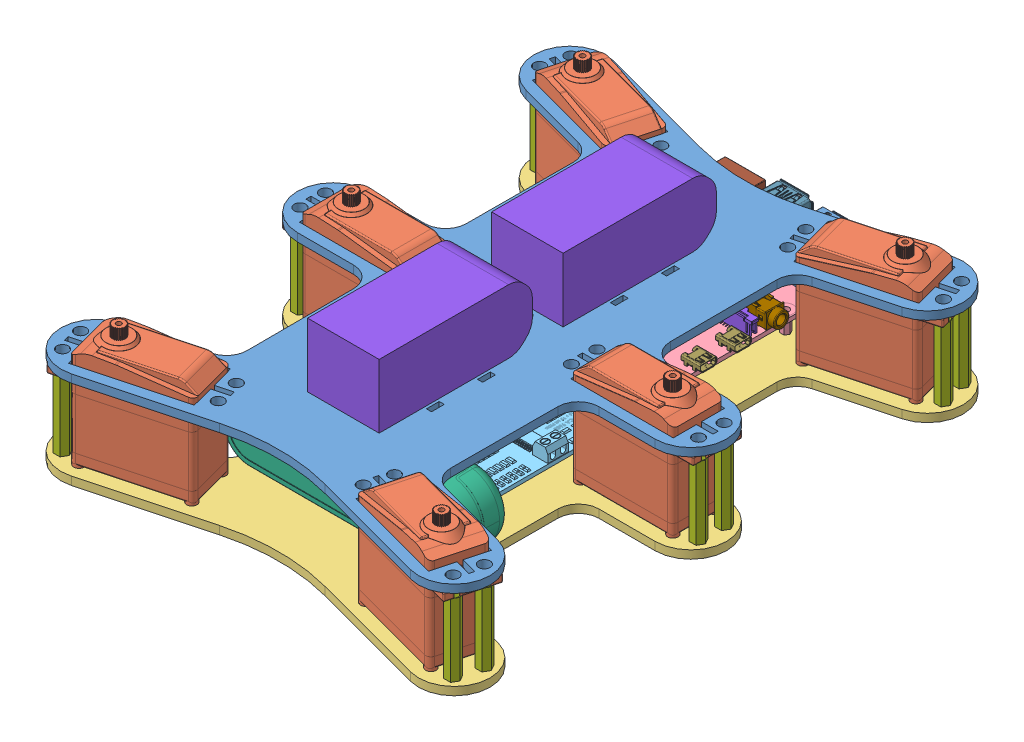
SolidWorks assembly BodyAssembly, configuration Default. Lengths in mm.
Overall size (168 62.85 216.72).
58 component instances, 26 part files, 52 mates.
Components (placement in the parent):
- TopPlate-1: TopPlate [Default] at (90.5661 120.22 158.5049) size (168 3.17 213.16)
- 20kg Servo-1: 20kg Servo [Default] at (37.0351 88.72 246.6736) x (-0.965926 0 0.258819) z (-0.258819 0 -0.965926) size (55.1 45.65 20.12)
- 20kg Servo-2: 20kg Servo [Default] at (37.6161 88.72 158.5049) x (-1 0 0) z (0 0 -1) size (55.1 45.65 20.12)
- 20kg Servo-3: 20kg Servo [Default] at (37.0351 88.72 70.3361) x (-0.965926 0 -0.258819) z (0.258819 0 -0.965926) size (55.1 45.65 20.12)
- 20kg Servo-4: 20kg Servo [Default] at (144.097 88.72 70.3361) x (0.965926 0 -0.258819) z (0.258819 0 0.965926) size (55.1 45.65 20.12)
- 20kg Servo-5: 20kg Servo [Default] at (143.5161 88.72 158.5049) size (55.1 45.65 20.12)
- 20kg Servo-6: 20kg Servo [Default] at (144.097 88.72 246.6736) x (0.965926 0 0.258819) z (-0.258819 0 0.965926) size (55.1 45.65 20.12)
- BottomBodyAssembly-1: BottomBodyAssembly [Default] at (-9.1402 -19.641 -5.3907) size (168 28.22 216.72)
  - BottomPlate-1: BottomPlate [Default] at (99.7063 105.186 163.8956) size (168 3.17 213.16)
  - Raspberry Pi 4 Model B-1: Raspberry Pi 4 Model B [Default] at (99.7063 115.161 100.2544) x (0 0 -1) z (1 0 0) size (88.99 19.9 58.4)
    - PCB, RPi4ModelB-1: PCB, RPi4ModelB [Default] at origin size (85 1.6 56)
    - Broadcom BCM2711B0 CPU, RPi4ModelB-1: Broadcom BCM2711B0 CPU, RPi4ModelB [Default] at (-13.25 0.8 -4.5) size (15 2.3 15)
    - 2.54 mm DUPONT MALE PIN HEADER, POE, 2X2, RPi4ModelB-1: 2.54 mm DUPONT MALE PIN HEADER, POE, 2X2, RPi4ModelB [Default] at (19 0.8 -18.5) size (5.08 11.3 5.08)
    - 2.54 mm DUPONT MALE PIN HEADER, IO, 2X20, RPi4ModelB-1: 2.54 mm DUPONT MALE PIN HEADER, IO, 2X20, RPi4ModelB [Default] at (-10 0.8 -24.5) size (50.8 11.3 5.08)
    - Camera Connector, RPi4ModelB-1: Camera Connector, RPi4ModelB [Default] at (4 0.8 16.5) x (0 0 -1) z (1 0 0) size (22.4 5.68 5.07)
    - Microphone Plug, RPi4ModelB-1: Microphone Plug, RPi4ModelB [Default] at (11.5 0.8 21.65) size (7.23 7.55 15)
    - Display Connector, RPi4ModelB-1: Display Connector, RPi4ModelB [Default] at (-38.5 0.8 0) x (0 0 1) z (-1 0 0) size (22.4 5.68 5.07)
    - Gigabit Ethernet Port, RPi4ModelB-1: Gigabit Ethernet Port, RPi4ModelB [Default] at (45.5 7.55 -17.75) x (0 0 -1) z (1 0 0) size (16.2 17.24 21.64)
    - Female Micro HDMI Connector, RPi4ModelB-2: Female Micro HDMI Connector, RPi4ModelB [Default] at (-3 0.8 27.3875) size (6.5 3.51 7.5)
    - Female Micro HDMI Connector, RPi4ModelB-3: Female Micro HDMI Connector, RPi4ModelB [Default] at (-16.5 0.8 27.3875) size (6.5 3.51 7.5)
    - Female USB Type C Connector, RPi4ModelB-1: Female USB Type C Connector, RPi4ModelB [Default] at (-31.3 0.8 26.5419) size (8.94 3.96 7.9)
    - 2X USB3.0 PORTS, RPi4ModelB-2: 2X USB3.0 PORTS, RPi4ModelB [Default] at (37.07 0.8 1) size (17.47 19.41 15.68)
    - 91D77 D9WHV 778K, 4 GB LPDDR4 SDRAM, RPi4ModelB-1: 91D77 D9WHV 778K, 4 GB LPDDR4 SDRAM, RPi4ModelB [Default] at (2.25 0.8 -4.5) size (10 0.8 14.5)
    - Cypress CYW43455 Wireless Module Cover, RPi4ModelB-1: Cypress CYW43455 Wireless Module Cover, RPi4ModelB [Default] at (-30.5 0.8 -14.5) size (11 1.6 13)
    - SD Card Slot, RPi4ModelB-1: SD Card Slot, RPi4ModelB [Default] at (-35.3 -0.8 0) x (0 0 -1) z (-1 0 0) size (11.95 1.45 11.4)
    - VIA VL805 PCIe USB 3.0 controller, RPi4ModelB-1: VIA VL805 PCIe USB 3.0 controller, RPi4ModelB [Default] at (17.5 0.8 4) size (8.8 0.8 8.8)
    - 2X USB2.0 PORTS, RPi4ModelB-1: 2X USB2.0 PORTS, RPi4ModelB [Default] at (37.065 0.65 19) size (17.87 19.16 15.33)
    - Broadcom BCM54213PE Gigabit Ethernet Transceiver, RPi4ModelB-1: Broadcom BCM54213PE Gigabit Ethernet Transceiver, RPi4ModelB [Default] at (16.5 0.8 -10) size (6.8 1 6.8)
    - MxL7704 Universal PMIC, RPi4ModelB-1: MxL7704 Universal PMIC, RPi4ModelB [Default] at (-32.5 0.8 16) size (5.4 0.8 5.4)
  - Pi Standoff-5: Pi Standoff [Default] at (72.6063 108.361 203.9544) size (3.46 6 3)
  - Pi Standoff-6: Pi Standoff [Default] at (91.4063 108.361 148.0544) size (3.46 6 3)
  - Pi Standoff-7: Pi Standoff [Default] at (108.0063 108.361 203.9544) size (3.46 6 3)
  - Pi Standoff-8: Pi Standoff [Default] at (91.4063 108.361 203.9544) size (3.46 6 3)
  - Pi Standoff-9: Pi Standoff [Default] at (72.6063 108.361 148.0544) size (3.46 6 3)
  - Pi Standoff-10: Pi Standoff [Default] at (126.8063 108.361 203.9544) size (3.46 6 3)
  - Pi Standoff-11: Pi Standoff [Default] at (126.8063 108.361 148.0544) size (3.46 6 3)
  - Pi Standoff-12: Pi Standoff [Default] at (108.0063 108.361 148.0544) size (3.46 6 3)
  - Pi Standoff-13: Pi Standoff [Default] at (75.2063 108.361 81.2544) size (3.46 6 3)
  - Pi Standoff-14: Pi Standoff [Default] at (75.2063 108.361 139.2544) size (3.46 6 3)
  - Pi Standoff-15: Pi Standoff [Default] at (124.2063 108.361 139.2544) size (3.46 6 3)
  - Pi Standoff-16: Pi Standoff [Default] at (124.2063 108.361 81.2544) size (3.46 6 3)
  - 12Channel PWM-1: 12Channel PWM [Default] at (82.0063 114.361 176.0044) size (25.4 9.51 66.7)
  - 12Channel PWM-2: 12Channel PWM [Default] at (117.4063 114.361 176.0044) size (25.4 9.51 66.7)
  - Intel Realsense D435-1: Intel Realsense D435 [Default] at (99.7063 120.861 213.7644) x (-1 0 0) z (0 1 0) size (90.24 25 25.08)
- ServoStandoffsBody-1: ServoStandoffsBody [Default] at (14.1328 88.72 257.9867) size (5.43 28.35 4.7)
- ServoStandoffsBody-2: ServoStandoffsBody [Default] at (11.5446 88.72 248.3274) size (5.43 28.35 4.7)
- ServoStandoffsBody-3: ServoStandoffsBody [Default] at (12.5661 88.72 163.5049) size (5.43 28.35 4.7)
- ServoStandoffsBody-4: ServoStandoffsBody [Default] at (12.5661 88.72 153.5049) size (5.43 28.35 4.7)
- ServoStandoffsBody-5: ServoStandoffsBody [Default] at (11.5446 88.72 68.6823) size (5.43 28.35 4.7)
- ServoStandoffsBody-6: ServoStandoffsBody [Default] at (166.9994 88.72 59.0231) size (5.43 28.35 4.7)
- ServoStandoffsBody-7: ServoStandoffsBody [Default] at (14.1328 88.72 59.0231) size (5.43 28.35 4.7)
- ServoStandoffsBody-8: ServoStandoffsBody [Default] at (166.9994 88.72 257.9867) size (5.43 28.35 4.7)
- ServoStandoffsBody-10: ServoStandoffsBody [Default] at (169.5876 88.72 248.3274) size (5.43 28.35 4.7)
- ServoStandoffsBody-11: ServoStandoffsBody [Default] at (168.5661 88.72 163.5049) size (5.43 28.35 4.7)
- ServoStandoffsBody-12: ServoStandoffsBody [Default] at (168.5661 88.72 153.5049) size (5.43 28.35 4.7)
- ServoStandoffsBody-13: ServoStandoffsBody [Default] at (169.5876 88.72 68.6823) size (5.43 28.35 4.7)
- LiPo Battery-1: LiPo Battery [Default] at (90.5661 123.395 194.5049) x (0 0 -1) z (1 0 0) size (60 25 28)
- LiPo Battery-2: LiPo Battery [Default] at (90.5661 123.395 122.5049) x (0 0 -1) z (1 0 0) size (60 25 28)
Mates (geometry in assembly coordinates):
- Concentric1: concentric anti-aligned: cylinder of TopPlate-1 through (11.5446 123.395 248.3274) axis (0 -1 0) radius 2.25; cylinder of 20kg Servo-1 through (11.5446 117.07 248.3274) axis (0 1 0) radius 2.075
- Concentric2: concentric anti-aligned: cylinder of TopPlate-1 through (14.1328 123.395 257.9867) axis (0 -1 0) radius 2.25; cylinder of 20kg Servo-1 through (14.1328 117.07 257.9867) axis (0 1 0) radius 2.075
- Coincident1: coincident anti-aligned: plane of TopPlate-1 through (20.5661 120.22 158.5049) normal (0 -1 0); plane of 20kg Servo-1 through (11.5446 120.22 248.3274) normal (0 1 0)
- Concentric3: concentric anti-aligned: cylinder of TopPlate-1 through (12.5661 123.395 153.5049) axis (0 -1 0) radius 2.25; cylinder of 20kg Servo-2 through (12.5661 117.07 153.5049) axis (0 1 0) radius 2.075
- Concentric4: concentric anti-aligned: cylinder of TopPlate-1 through (12.5661 123.395 163.5049) axis (0 -1 0) radius 2.25; cylinder of 20kg Servo-2 through (12.5661 117.07 163.5049) axis (0 1 0) radius 2.075
- Coincident2: coincident anti-aligned: plane of TopPlate-1 through (20.5661 120.22 158.5049) normal (0 -1 0); plane of 20kg Servo-2 through (12.5661 120.22 153.5049) normal (0 1 0)
- Coincident3: coincident anti-aligned: plane of TopPlate-1 through (20.5661 120.22 158.5049) normal (0 -1 0); plane of 20kg Servo-3 through (14.1328 120.22 59.0231) normal (0 1 0)
- Concentric5: concentric anti-aligned: cylinder of TopPlate-1 through (11.5446 123.395 68.6823) axis (0 -1 0) radius 2.25; cylinder of 20kg Servo-3 through (11.5446 117.07 68.6823) axis (0 1 0) radius 2.075
- Concentric6: concentric anti-aligned: cylinder of TopPlate-1 through (14.1328 123.395 59.0231) axis (0 -1 0) radius 2.25; cylinder of 20kg Servo-3 through (14.1328 117.07 59.0231) axis (0 1 0) radius 2.075
- Concentric7: concentric anti-aligned: cylinder of TopPlate-1 through (166.9994 123.395 257.9867) axis (0 -1 0) radius 2.25; cylinder of 20kg Servo-6 through (166.9994 117.07 257.9867) axis (0 1 0) radius 2.075
- Concentric8: concentric anti-aligned: cylinder of TopPlate-1 through (169.5876 123.395 248.3274) axis (0 -1 0) radius 2.25; cylinder of 20kg Servo-6 through (169.5876 117.07 248.3274) axis (0 1 0) radius 2.075
- Coincident4: coincident anti-aligned: plane of TopPlate-1 through (20.5661 120.22 158.5049) normal (0 -1 0); plane of 20kg Servo-6 through (166.9994 120.22 257.9867) normal (0 1 0)
- Concentric10: concentric anti-aligned: cylinder of TopPlate-1 through (168.5661 123.395 163.5049) axis (0 -1 0) radius 2.25; cylinder of 20kg Servo-5 through (168.5661 117.07 163.5049) axis (0 1 0) radius 2.075
- Concentric11: concentric anti-aligned: cylinder of TopPlate-1 through (168.5661 123.395 153.5049) axis (0 -1 0) radius 2.25; cylinder of 20kg Servo-5 through (168.5661 117.07 153.5049) axis (0 1 0) radius 2.075
- Coincident5: coincident anti-aligned: plane of TopPlate-1 through (20.5661 120.22 158.5049) normal (0 -1 0); plane of 20kg Servo-5 through (168.5661 120.22 163.5049) normal (0 1 0)
- Concentric12: concentric anti-aligned: cylinder of TopPlate-1 through (166.9994 123.395 59.0231) axis (0 -1 0) radius 2.25; cylinder of 20kg Servo-4 through (166.9994 117.07 59.0231) axis (0 1 0) radius 2.075
- Concentric13: concentric anti-aligned: cylinder of TopPlate-1 through (169.5876 123.395 68.6823) axis (0 -1 0) radius 2.25; cylinder of 20kg Servo-4 through (169.5876 117.07 68.6823) axis (0 1 0) radius 2.075
- Coincident6: coincident anti-aligned: plane of TopPlate-1 through (20.5661 120.22 158.5049) normal (0 -1 0); plane of 20kg Servo-4 through (169.5876 120.22 68.6823) normal (0 1 0)
- Concentric14: concentric aligned: cylinder of TopPlate-1 through (90.5661 123.395 329.646) axis (0 1 0) radius 80; cylinder of BottomBodyAssembly-1/BottomPlate-1 through (90.5661 88.72 329.646) axis (0 1 0) radius 80
- Coincident8: coincident anti-aligned: plane of 20kg Servo-1 through (37.0351 88.72 246.6736) normal (0 -1 0); plane of BottomBodyAssembly-1/BottomPlate-1 through (20.5661 88.72 158.5049) normal (0 1 0)
- Coincident9: coincident aligned: plane of TopPlate-1 through (50.5661 123.395 172.5049) normal (-0.999995 0 0.003285); plane of BottomBodyAssembly-1/BottomPlate-1 through (50.5661 88.72 172.5049) normal (-0.999995 0 0.003285)
- Concentric16: concentric aligned: cylinder of TopPlate-1 through (14.1328 123.395 257.9867) axis (0 -1 0) radius 2.25; cylinder of ServoStandoffsBody-1 through (14.1328 117.07 257.9867) axis (0 -1 0) radius 2.25
- Coincident12: coincident anti-aligned: plane of BottomBodyAssembly-1/BottomPlate-1 through (20.5661 88.72 158.5049) normal (0 1 0); plane of ServoStandoffsBody-1 through (14.1328 88.72 257.9867) normal (0 -1 0)
- Concentric17: concentric aligned: cylinder of TopPlate-1 through (11.5446 123.395 248.3274) axis (0 -1 0) radius 2.25; cylinder of ServoStandoffsBody-2 through (11.5446 117.07 248.3274) axis (0 -1 0) radius 2.25
- Coincident13: coincident aligned: plane of BottomBodyAssembly-1/BottomPlate-1 through (20.5661 88.72 158.5049) normal (0 1 0); circle of ServoStandoffsBody-2
- Concentric18: concentric aligned: cylinder of TopPlate-1 through (12.5661 123.395 163.5049) axis (0 -1 0) radius 2.25; cylinder of ServoStandoffsBody-3 through (12.5661 117.07 163.5049) axis (0 -1 0) radius 2.25
- Coincident14: coincident aligned: plane of BottomBodyAssembly-1/BottomPlate-1 through (20.5661 88.72 158.5049) normal (0 1 0); circle of ServoStandoffsBody-3
- Concentric19: concentric aligned: cylinder of TopPlate-1 through (12.5661 123.395 153.5049) axis (0 -1 0) radius 2.25; cylinder of ServoStandoffsBody-4 through (12.5661 117.07 153.5049) axis (0 -1 0) radius 2.25
- Coincident15: coincident aligned: plane of BottomBodyAssembly-1/BottomPlate-1 through (20.5661 88.72 158.5049) normal (0 1 0); circle of ServoStandoffsBody-4
- Concentric20: concentric aligned: cylinder of TopPlate-1 through (11.5446 123.395 68.6823) axis (0 -1 0) radius 2.25; cylinder of ServoStandoffsBody-5 through (11.5446 117.07 68.6823) axis (0 -1 0) radius 2.25
- Coincident16: coincident aligned: plane of BottomBodyAssembly-1/BottomPlate-1 through (20.5661 88.72 158.5049) normal (0 1 0); circle of ServoStandoffsBody-5
- Concentric21: concentric aligned: cylinder of TopPlate-1 through (14.1328 123.395 59.0231) axis (0 -1 0) radius 2.25; cylinder of ServoStandoffsBody-7 through (14.1328 117.07 59.0231) axis (0 -1 0) radius 2.25
- Coincident17: coincident aligned: plane of BottomBodyAssembly-1/BottomPlate-1 through (20.5661 88.72 158.5049) normal (0 1 0); circle of ServoStandoffsBody-7
- Concentric22: concentric aligned: cylinder of TopPlate-1 through (166.9994 123.395 59.0231) axis (0 -1 0) radius 2.25; cylinder of ServoStandoffsBody-6 through (166.9994 117.07 59.0231) axis (0 -1 0) radius 2.25
- Coincident18: coincident aligned: plane of BottomBodyAssembly-1/BottomPlate-1 through (20.5661 88.72 158.5049) normal (0 1 0); circle of ServoStandoffsBody-6
- Concentric23: concentric aligned: cylinder of TopPlate-1 through (169.5876 123.395 68.6823) axis (0 -1 0) radius 2.25; cylinder of ServoStandoffsBody-13 through (169.5876 117.07 68.6823) axis (0 -1 0) radius 2.25
- Coincident19: coincident aligned: plane of BottomBodyAssembly-1/BottomPlate-1 through (20.5661 88.72 158.5049) normal (0 1 0); circle of ServoStandoffsBody-13
- Concentric24: concentric aligned: cylinder of TopPlate-1 through (168.5661 123.395 153.5049) axis (0 -1 0) radius 2.25; cylinder of ServoStandoffsBody-12 through (168.5661 117.07 153.5049) axis (0 -1 0) radius 2.25
- Coincident20: coincident aligned: plane of BottomBodyAssembly-1/BottomPlate-1 through (20.5661 88.72 158.5049) normal (0 1 0); circle of ServoStandoffsBody-12
- Concentric25: concentric aligned: cylinder of TopPlate-1 through (168.5661 123.395 163.5049) axis (0 -1 0) radius 2.25; cylinder of ServoStandoffsBody-11 through (168.5661 117.07 163.5049) axis (0 -1 0) radius 2.25
- Coincident21: coincident aligned: plane of BottomBodyAssembly-1/BottomPlate-1 through (20.5661 88.72 158.5049) normal (0 1 0); circle of ServoStandoffsBody-11
- Concentric26: concentric aligned: cylinder of TopPlate-1 through (169.5876 123.395 248.3274) axis (0 -1 0) radius 2.25; cylinder of ServoStandoffsBody-10 through (169.5876 117.07 248.3274) axis (0 -1 0) radius 2.25
- Coincident22: coincident aligned: plane of BottomBodyAssembly-1/BottomPlate-1 through (20.5661 88.72 158.5049) normal (0 1 0); circle of ServoStandoffsBody-10
- Concentric27: concentric aligned: cylinder of TopPlate-1 through (166.9994 123.395 257.9867) axis (0 -1 0) radius 2.25; cylinder of ServoStandoffsBody-8 through (166.9994 117.07 257.9867) axis (0 -1 0) radius 2.25
- Coincident23: coincident aligned: plane of BottomBodyAssembly-1/BottomPlate-1 through (20.5661 88.72 158.5049) normal (0 1 0); circle of ServoStandoffsBody-8
- Width1: width anti-aligned: plane of TopPlate-1 through (130.5661 123.395 172.5049) normal (0.999995 0 0.003285); plane of LiPo Battery-1 through (50.5661 123.395 172.5049) normal (-0.999995 0 0.003285); plane of TopPlate-1 through (104.5661 148.395 224.5049) normal (1 0 0); plane of LiPo Battery-1 through (76.5661 148.395 224.5049) normal (-1 0 0)
- Coincident24: coincident aligned: plane of LiPo Battery-1 through (76.5661 148.395 224.5049) normal (-1 0 0); plane of LiPo Battery-2 through (76.5661 148.395 152.5049) normal (-1 0 0)
- Coincident25: coincident aligned: plane of LiPo Battery-1 through (104.5661 148.395 224.5049) normal (1 0 0); plane of LiPo Battery-2 through (104.5661 148.395 152.5049) normal (1 0 0)
- Coincident26: coincident anti-aligned: plane of TopPlate-1 through (20.5661 123.395 158.5049) normal (0 1 0); plane of LiPo Battery-1 through (90.5661 123.395 194.5049) normal (0 -1 0)
- Coincident27: coincident aligned: plane of LiPo Battery-1 through (90.5661 148.395 194.5049) normal (0 1 0); plane of LiPo Battery-2 through (90.5661 148.395 122.5049) normal (0 1 0)
- Distance1: distance = 12 mm anti-aligned: plane of LiPo Battery-2 through (76.5661 148.395 152.5049) normal (0 0 1); plane of LiPo Battery-1 through (76.5661 148.395 164.5049) normal (0 0 -1)
- Width2: width anti-aligned: plane of LiPo Battery-1 through (76.5661 148.395 224.5049) normal (0 0 1); plane of TopPlate-1 through (76.5661 148.395 92.5049) normal (0 0 -1); plane of LiPo Battery-2 through (160.5661 123.395 144.5049) normal (0 0 -1); plane of TopPlate-1 through (160.5661 123.395 172.5049) normal (0 0 1)
